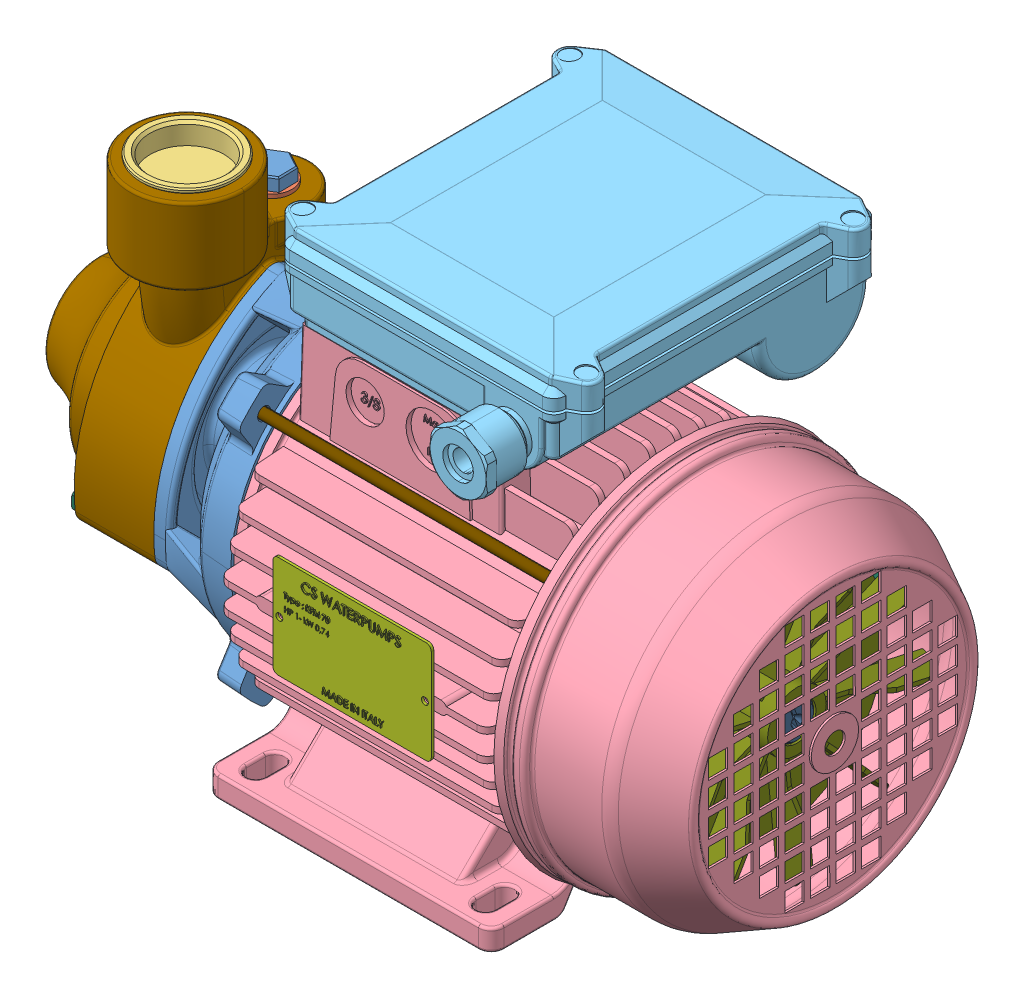
SolidWorks assembly Elettropompa KF  Inox, configuration Default. Lengths in mm.
Overall size (290.35 207.83 196.66).
68 component instances, 35 part files, 71 mates.
Components (placement in the parent):
- Supporto motore KF 65_70-1: Supporto motore KF 65_70 [Default] at (-54.2626 10.5524 119.1659) x (0 0 1) z (-1 0 0) size (120 120 55)
- Gruppo statore avvolto H80 con carcassa  B3 e portacondensatore-1: Gruppo statore avvolto H80 con carcassa  B3 e portacondensatore [Default] at (62.7261 5.2741 9.1659) size (151.55 207.83 196.66)
  - Statore 110x55H70-1: Statore 110x55H70 [Default] at (-35.1887 5.2783 110) x (0 0 -1) z (1 0 0) size (110 110 80)
  - corona avvolgimeno-1: corona avvolgimeno [Default] at (-75.1887 5.2783 110) x (0 -0.91858 0.395234) z (0 -0.395234 -0.91858) size (95 25 95)
  - corona avvolgimeno-2: corona avvolgimeno [Default] at (4.8113 5.2783 110) x (0 0.057001 0.998374) z (0 0.998374 -0.057001) size (95 25 95)
  - Carcassa MEC 71 B3-1: Carcassa MEC 71 B3 [Default] at (14.0613 5.2783 110) x (0 0 1) z (-1 0 0) size (140 148 121.5)
  - COPRIMORS_MEC63-71_MONOFASE_M4-1: COPRIMORS_MEC63-71_MONOFASE_M4 [Default] at (-55.6887 85.2783 110) x (-1 0 0) z (0 0 -1) size (121.11 50.5 148)
  - Calotta MEC 71 Lavorata-1: Calotta MEC 71 Lavorata [Default] at (15.8113 5.2783 110) x (0 -0.70802 -0.706193) z (0 -0.706193 0.70802) size (139.06 30 139.06)
  - targhetta metallica-1: targhetta metallica [Default] at (-10.1875 -9.7179 181) x (-1 -0.000063 0) z (0 0 -1) size (62 40 1.5)
- Girante cod KFM 65_70-1: Girante cod KFM 65_70 [Default] at (-95.8876 10.5524 119.1659) x (0 0.937754 0.347301) z (-1 0 0) size (70.8 70.8 15.13)
- Corpo pompa KF 65_70-1: Corpo pompa KF 65_70 [Default] at (-96.0626 10.5524 119.1659) x (0 0 1) z (-1 0 0) size (93.39 132.5 74.65)
- Assieme9-1: Assieme9 [Default] at (49.0791 -228.781 32.0447) x (1 0 0) z (0 0.937754 0.347301) size (231.8 61.88 61.88)
  - Albero KF 70-1: Albero KF 70 [Default] at (75.6583 1.4226 254.6931) x (-1 0 0) z (0 0 -1) size (231.8 17 17)
  - SKF_W_6202_2RS1-1: SKF_W_6202_2RS1 [Default] at (38.6583 1.4226 254.6931) x (1 0 0) z (0 -0.991359 0.13118) size (11 35 35)
    - SKF_W_6202_2RS1_12-1: SKF_W_6202_2RS1_12 [Default] x (1 0 0) z (0 -0.707107 0.707107) size (5.95 5.95 5.95)
    - SKF_W_6202_2RS1_12-2: SKF_W_6202_2RS1_12 [Default] x (1 0 0) z (0 -1 0) size (5.95 5.95 5.95)
    - SKF_W_6202_2RS1_12-3: SKF_W_6202_2RS1_12 [Default] x (1 0 0) z (0 -0.707107 -0.707107) size (5.95 5.95 5.95)
    - SKF_W_6202_2RS1_12-4: SKF_W_6202_2RS1_12 [Default] x (1 0 0) z (0 0 -1) size (5.95 5.95 5.95)
    - SKF_W_6202_2RS1_12-5: SKF_W_6202_2RS1_12 [Default] x (1 0 0) z (0 0.707107 -0.707107) size (5.95 5.95 5.95)
    - SKF_W_6202_2RS1_12-6: SKF_W_6202_2RS1_12 [Default] x (1 0 0) z (0 1 0) size (5.95 5.95 5.95)
    - SKF_W_6202_2RS1_12-7: SKF_W_6202_2RS1_12 [Default] x (1 0 0) z (0 0.707107 0.707107) size (5.95 5.95 5.95)
    - SKF_W_6202_2RS1_12-8: SKF_W_6202_2RS1_12 [Default] at origin size (5.95 5.95 5.95)
    - SKF_W_6202_2RS1_21-1: SKF_W_6202_2RS1_21 [Default] at origin size (11 35 35)
    - SKF_W_6202_2RS1_23-1: SKF_W_6202_2RS1_23 [Default] at origin size (11 31.4 31.4)
  - SKF_W_6202_2RS1-2: SKF_W_6202_2RS1 [Default] at (-103.3417 1.4226 254.6931) x (1 0 0) z (0 -0.849888 -0.526963) size (11 35 35)
    - SKF_W_6202_2RS1_12-1: SKF_W_6202_2RS1_12 [Default] x (1 0 0) z (0 -0.707107 0.707107) size (5.95 5.95 5.95)
    - SKF_W_6202_2RS1_12-2: SKF_W_6202_2RS1_12 [Default] x (1 0 0) z (0 -1 0) size (5.95 5.95 5.95)
    - SKF_W_6202_2RS1_12-3: SKF_W_6202_2RS1_12 [Default] x (1 0 0) z (0 -0.707107 -0.707107) size (5.95 5.95 5.95)
    - SKF_W_6202_2RS1_12-4: SKF_W_6202_2RS1_12 [Default] x (1 0 0) z (0 0 -1) size (5.95 5.95 5.95)
    - SKF_W_6202_2RS1_12-5: SKF_W_6202_2RS1_12 [Default] x (1 0 0) z (0 0.707107 -0.707107) size (5.95 5.95 5.95)
    - SKF_W_6202_2RS1_12-6: SKF_W_6202_2RS1_12 [Default] x (1 0 0) z (0 1 0) size (5.95 5.95 5.95)
    - SKF_W_6202_2RS1_12-7: SKF_W_6202_2RS1_12 [Default] x (1 0 0) z (0 0.707107 0.707107) size (5.95 5.95 5.95)
    - SKF_W_6202_2RS1_12-8: SKF_W_6202_2RS1_12 [Default] at origin size (5.95 5.95 5.95)
    - SKF_W_6202_2RS1_21-1: SKF_W_6202_2RS1_21 [Default] at origin size (11 35 35)
    - SKF_W_6202_2RS1_23-1: SKF_W_6202_2RS1_23 [Default] at origin size (11 31.4 31.4)
  - Rotore-1: Rotore [90] at (-20.3417 1.4226 254.6931) x (1 0 0) z (0 -0.148651 0.98889) size (88 54.4 54.4)
  - Chiavetta 4x4x10-1: Chiavetta 4x4x10 [Default] at (-148.1417 8.4226 254.6931) x (1 0 0) z (0 -1 0) size (10 4 3.8)
- Ventola MEC71  FORO 15-1: Ventola MEC71  FORO 15 [Default] at (-99.6626 10.5524 119.1659) x (0 -0.861898 0.507081) z (1 0 0) size (127 121.28 15.42)
- Rompigoccia-1: Rompigoccia [Default] at (-54.2626 10.5524 119.1659) x (0 0 1) z (0 -1 0) size (33.06 8 33.06)
- tirante  5x135-1: tirante  5x135 [Default] at (86.5374 55.5524 164.1659) x (-1 0 0) z (0 0 -1) size (137.41 8.1 7.02)
- tirante  5x135-2: tirante  5x135 [Default] at (86.5374 -34.4476 164.1659) x (-1 0 0) z (0 -0.8306 -0.556869) size (137.41 8.1 7.02)
- tirante  5x135-3: tirante  5x135 [Default] at (86.5374 55.5524 74.1659) x (-1 0 0) z (0 -0.008382 -0.999965) size (137.41 8.1 7.02)
- tirante  5x135-4: tirante  5x135 [Default] at (86.5374 -34.4476 74.1659) x (-1 0 0) z (0 -0.959675 -0.281111) size (137.41 8.1 7.02)
- tappo 1_8-1: tappo 1_8 [Default] at (-96.0626 77.0524 104.1659) x (-1 0 0) z (0 1 0) size (13.16 15.01 12)
- Rondella alluminio 1_8-1: Rondella alluminio 1_8 [Default] at (-96.0626 75.5524 104.1659) size (16 1.5 16)
- Tappo salvafiletto 1 pollice-1: Tappo salvafiletto 1 pollice [Default] at (-140.7406 10.5524 119.1659) x (-1 0 0) z (0 0.938506 0.345262) size (9.54 36.1 36.1)
- Tappo salvafiletto 1 pollice-2: Tappo salvafiletto 1 pollice [Default] at (-96.0626 92.8304 137.1659) x (0 1 0) z (0.026176 0 -0.999657) size (9.54 36.1 36.1)
- Copriventola MEC 71-1: Copriventola MEC 71 [Default] at (77.5374 10.5524 119.1659) x (-1 0 0) z (0 -0.000219 1) size (62.53 143.02 143.02)
- morsettiera-1: morsettiera [Default] at (30.5627 41.122 115.2906) x (0 0 1) z (0 1 0) size (27 42 19.32)
  - base morsettiera-1: base morsettiera [Default] at (3.8753 -23.6462 42.9304) x (-1 0 0) z (0 0 -1) size (27 42 10.5)
  - perno morsettiera-1: perno morsettiera [Default] at (11.8753 -39.1462 42.6304) size (4.5 4.63 11.12)
  - perno morsettiera-2: perno morsettiera [Default] at (-4.1247 -39.1462 42.6304) size (4.5 4.63 11.12)
  - perno morsettiera-3: perno morsettiera [Default] at (11.8753 -8.1462 42.6304) size (4.5 4.63 11.12)
- STAZIONARIA-2: STAZIONARIA [Default] at (-71.4228 -14.1935 127.8022) x (0 -0.44605 -0.895008) z (0 0.895008 -0.44605) size (26 8 26)
  - GOMMA-1: GOMMA [Default] at (-3.3084 -4.4601 26) size (26 7 26)
  - CERAMICA-1: CERAMICA [Default] at (-3.3084 -0.9601 26) x (0.999975 0 0.00709) z (-0.00709 0 0.999975) size (22 4.5 22)
- ROTANTE-1: ROTANTE [Default] at (-75.2954 30.2911 126.3816) x (0 -0.30619 0.951971) z (0 -0.951971 -0.30619) size (32.11 13 32.11)
  - Parte4-1: Parte4 [Default] at (-0.8254 8.0815 21) size (21 3.5 21)
  - Parte5-1: Parte5 [Default] at (-0.8254 1.4673 21) size (24 8.4 24)
  - Parte6-1: Parte6 [Default] at (-0.8254 -0.3327 21) size (23 5 23)
  - Parte7-1: Parte7 [Default] at (-0.8254 4.6673 21) size (23 8 23)
  - Parte8-1: Parte8 [Default] at (-0.8254 5.6673 21) x (0.584934 0 0.811081) z (-0.811081 0 0.584934) size (23 1 23)
  - Parte2-2: Parte2 [Default] at (-0.5063 7.2427 20.915) x (-1 0 0) z (0 1 0) size (21.2 21.25 5.09)
- 621015x35-1: 621015x35 [Default] at (-111.6626 57.0524 119.1659) size (38.51 9.26 8.02)
- 621015x35-2: 621015x35 [Default] at (-111.6626 -12.6976 159.4361) size (38.51 9.26 8.02)
- 621015x35-3: 621015x35 [Default] at (-111.6626 -12.6976 78.8957) size (38.51 9.26 8.02)
- 10_00_0471_0120_002-1: 10_00_0471_0120_002 [Default] at (-89.0626 10.46 119.5551) x (0 -0.972953 -0.231005) z (1 0 0) size (14.3 16.3 1)
- Rondella tenuta-1: Rondella tenuta [Default] at (-88.0626 10.5524 119.1659) x (0 0 -1) z (0 -1 0) size (21 0.1 21)
Mates (geometry in assembly coordinates):
- Concentrico1: concentric aligned: cylinder of Supporto motore KF 65_70-1 through (-54.2626 10.5524 119.1659) axis (1 0 0) radius 56.9; cylinder of Gruppo statore avvolto H80 con carcassa  B3 e portacondensatore-1/Carcassa MEC 71 B3-1 through (-39.9626 10.5524 119.1659) axis (1 0 0) radius 57
- Coincidente1: coincident anti-aligned: plane of Supporto motore KF 65_70-1 through (-36.9626 67.4524 119.1659) normal (1 0 0); plane of Gruppo statore avvolto H80 con carcassa  B3 e portacondensatore-1/Carcassa MEC 71 B3-1 through (-36.9626 10.5524 119.1659) normal (-1 0 0)
- Concentrico2: concentric anti-aligned: circle of Supporto motore KF 65_70-1; circle of Girante cod KFM 65_70-1
- Distanza1: distance = 0.05 mm anti-aligned: plane of Girante cod KFM 65_70-1 through (-92.0126 18.9571 96.4723) normal (1 0 0); plane of Supporto motore KF 65_70-1 through (-91.9626 35.7524 119.1659) normal (-1 0 0)
- Concentrico3: concentric aligned: cylinder of Supporto motore KF 65_70-1 through (-54.2626 10.5524 119.1659) axis (1 0 0) radius 35.45; cylinder of Corpo pompa KF 65_70-1 through (-104.2626 10.5524 119.1659) axis (1 0 0) radius 35.5
- Coincidente3: coincident anti-aligned: plane of Supporto motore KF 65_70-1 through (-80.4626 63.0524 119.1659) normal (-1 0 0); plane of Corpo pompa KF 65_70-1 through (-80.4626 -8.9027 125.7387) normal (1 0 0)
- Coincidente4: coincident anti-aligned: plane of Supporto motore KF 65_70-1 through (-54.2626 23.0524 119.1659) normal (1 0 0); plane of Assieme9-1/SKF_W_6202_2RS1-2/SKF_W_6202_2RS1_21-1 through (-54.2626 20.9285 132.5055) normal (-1 0 0)
- Concentrico4: concentric aligned: cylinder of Supporto motore KF 65_70-1 through (-54.2626 10.5524 119.1659) axis (1 0 0) radius 17.5; cylinder of Assieme9-1/SKF_W_6202_2RS1-2/SKF_W_6202_2RS1_21-1 through (-4.2626 10.5524 119.1659) axis (1 0 0) radius 17.5
- Coincidente5: coincident anti-aligned: plane of Girante cod KFM 65_70-1 through (-92.0126 11.4727 110.9224) normal (0 0.937754 0.347301); plane of Assieme9-1/Chiavetta 4x4x10-1 through (-102.0626 9.7883 115.4705) normal (0 -0.937754 -0.347301)
- Concentrico5: concentric aligned: circle of Gruppo statore avvolto H80 con carcassa  B3 e portacondensatore-1/Calotta MEC 71 Lavorata-1; cylinder of Ventola MEC71  FORO 15-1 through (124.7374 10.5524 119.1659) axis (1 0 0) radius 7.5
- Coincidente6: coincident aligned: plane of Assieme9-1/Albero KF 70-1 through (124.7374 10.5524 119.1659) normal (1 0 0); plane of Ventola MEC71  FORO 15-1 through (124.7374 10.5524 119.1659) normal (1 0 0)
- Blocca1: lock: unknown of Assieme9-1/Albero KF 70-1; unknown of Ventola MEC71  FORO 15-1
- Concentrico6: concentric anti-aligned: cylinder of Assieme9-1/Albero KF 70-1 through (124.7374 10.5524 119.1659) axis (1 0 0) radius 6; cylinder of Rompigoccia-1 through (-97.7632 10.5524 119.1659) axis (-1 0 0) radius 6
- Coincidente7: coincident anti-aligned: plane of Assieme9-1/Albero KF 70-1 through (-54.2626 12.6363 113.5394) normal (-1 0 0); plane of Rompigoccia-1 through (-54.2626 10.5524 113.1659) normal (1 0 0)
- Concentrico7: concentric anti-aligned: cylinder of Supporto motore KF 65_70-1 through (-38.9626 55.5524 164.1659) axis (1 0 0) radius 2.1; cylinder of tirante  5x135-1 through (86.9374 55.5524 164.1659) axis (-1 0 0) radius 2
- Coincidente8: coincident anti-aligned: plane of Gruppo statore avvolto H80 con carcassa  B3 e portacondensatore-1/Calotta MEC 71 Lavorata-1 through (86.5374 59.7806 168.267) normal (1 0 0); plane of tirante  5x135-1 through (86.5374 57.5524 164.1659) normal (-1 0 0)
- Concentrico8: concentric anti-aligned: cylinder of Supporto motore KF 65_70-1 through (-38.9626 -34.4476 164.1659) axis (1 0 0) radius 2.1; cylinder of tirante  5x135-2 through (86.9374 -34.4476 164.1659) axis (-1 0 0) radius 2
- Coincidente10: coincident anti-aligned: plane of Gruppo statore avvolto H80 con carcassa  B3 e portacondensatore-1/Calotta MEC 71 Lavorata-1 through (86.5374 -38.5487 168.3941) normal (1 0 0); plane of tirante  5x135-2 through (86.5374 -33.3338 162.5047) normal (-1 0 0)
- Concentrico9: concentric anti-aligned: cylinder of Supporto motore KF 65_70-1 through (-38.9626 55.5524 74.1659) axis (1 0 0) radius 2.1; cylinder of tirante  5x135-3 through (86.9374 55.5524 74.1659) axis (-1 0 0) radius 2
- Coincidente11: coincident anti-aligned: plane of Gruppo statore avvolto H80 con carcassa  B3 e portacondensatore-1/Calotta MEC 71 Lavorata-1 through (86.5374 59.6536 69.9377) normal (1 0 0); plane of tirante  5x135-3 through (86.5374 57.5524 74.1491) normal (-1 0 0)
- Concentrico10: concentric anti-aligned: cylinder of Supporto motore KF 65_70-1 through (-38.9626 -34.4476 74.1659) axis (1 0 0) radius 2.1; cylinder of tirante  5x135-4 through (86.9374 -34.4476 74.1659) axis (-1 0 0) radius 2
- Coincidente12: coincident anti-aligned: plane of Gruppo statore avvolto H80 con carcassa  B3 e portacondensatore-1/Calotta MEC 71 Lavorata-1 through (86.5374 -38.6758 70.0647) normal (1 0 0); plane of tirante  5x135-4 through (86.5374 -33.8853 72.2465) normal (-1 0 0)
- Parallelo2: parallel anti-aligned: plane of Gruppo statore avvolto H80 con carcassa  B3 e portacondensatore-1/Carcassa MEC 71 B3-1 through (-36.9626 -59.4476 74.3349) normal (0 -1 0); plane of Corpo pompa KF 65_70-1 through (-96.0626 100.5524 137.1659) normal (0 1 0)
- Concentrico121: concentric anti-aligned: cylinder of Corpo pompa KF 65_70-1 through (-111.6626 57.0524 119.1659) axis (1 0 0) radius 2.75; cylinder of hex bolt gradeab_iso-1 through (-115.1626 57.0495 118.6437) axis (-1 0 0) radius 4
- Coincidente141: coincident anti-aligned: plane of Corpo pompa KF 65_70-1 through (-111.6626 -8.9027 125.7387) normal (-1 0 0); plane of hex bolt gradeab_iso-1 through (-111.6626 61.6683 118.6437) normal (1 0 0)
- Concentrico13: concentric anti-aligned: cylinder of Corpo pompa KF 65_70-1 through (-111.6626 -12.6976 159.4361) axis (1 0 0) radius 2.75; cylinder of hex bolt gradeab_iso-2 through (-115.1626 -10.3429 160.7067) axis (-1 0 0) radius 4
- Coincidente15: coincident anti-aligned: plane of Corpo pompa KF 65_70-1 through (-111.6626 -8.9027 125.7387) normal (-1 0 0); plane of hex bolt gradeab_iso-2 through (-111.6626 -5.7241 160.7067) normal (1 0 0)
- Concentrico14: concentric anti-aligned: cylinder of Corpo pompa KF 65_70-1 through (-111.6626 -12.6976 78.8957) axis (1 0 0) radius 6; cylinder of hex bolt gradeab_iso-3 through (-115.1626 -14.9753 80.2996) axis (-1 0 0) radius 4
- Coincidente16: coincident anti-aligned: plane of Corpo pompa KF 65_70-1 through (-111.6626 -8.9027 125.7387) normal (-1 0 0); plane of hex bolt gradeab_iso-3 through (-111.6626 -10.3565 80.2996) normal (1 0 0)
- Concentrico15: concentric anti-aligned: cylinder of Corpo pompa KF 65_70-1 through (-111.6626 57.0524 119.1659) axis (1 0 0) radius 2.75; cylinder of hex bolt gradeab_iso-4 through (-115.1626 56.9755 116.4914) axis (-1 0 0) radius 4
- Coincidente17: coincident anti-aligned: plane of Corpo pompa KF 65_70-1 through (-111.6626 -8.9027 125.7387) normal (-1 0 0); plane of hex bolt gradeab_iso-4 through (-111.6626 61.5943 116.4914) normal (1 0 0)
- Concentrico16: concentric anti-aligned: cylinder of Corpo pompa KF 65_70-1 through (-111.6626 -12.6976 159.4361) axis (1 0 0) radius 2.75; cylinder of hex bolt gradeab_iso-5 through (-115.1626 -10.3429 160.7067) axis (-1 0 0) radius 4
- Coincidente18: coincident anti-aligned: plane of Corpo pompa KF 65_70-1 through (-111.6626 -8.9027 125.7387) normal (-1 0 0); plane of hex bolt gradeab_iso-5 through (-111.6626 -5.7241 160.7067) normal (1 0 0)
- Concentrico17: concentric: cylinder of Corpo pompa KF 65_70-1 through (-111.6626 -12.6976 78.8957) axis (1 0 0) radius 2.75; cylinder of hex bolt gradeab_iso-6 through (-115.1626 -14.9753 80.2996) axis (-1 0 0) radius 4
- Coincidente19: coincident anti-aligned: plane of Corpo pompa KF 65_70-1 through (-111.6626 -8.9027 125.7387) normal (-1 0 0); plane of hex bolt gradeab_iso-6 through (-111.6626 -10.3565 80.2996) normal (1 0 0)
- Concentrico18: concentric anti-aligned: cylinder of Corpo pompa KF 65_70-1 through (-111.6626 57.0524 119.1659) axis (1 0 0) radius 2.75; cylinder of hex bolt gradeab_iso-7 through (-115.1626 57.0524 119.1659) axis (-1 0 0) radius 4
- Coincidente20: coincident anti-aligned: plane of Corpo pompa KF 65_70-1 through (-111.6626 -8.9027 125.7387) normal (-1 0 0); plane of hex bolt gradeab_iso-7 through (-111.6626 61.1206 116.9788) normal (1 0 0)
- Concentrico19: concentric anti-aligned: cylinder of Corpo pompa KF 65_70-1 through (-111.6626 -12.6976 159.4361) axis (1 0 0) radius 6; cylinder of hex bolt gradeab_iso-8 through (-115.1626 -12.6976 159.4361) axis (-1 0 0) radius 4
- Coincidente21: coincident anti-aligned: plane of Corpo pompa KF 65_70-1 through (-111.6626 -8.9027 125.7387) normal (-1 0 0); plane of hex bolt gradeab_iso-8 through (-111.6626 -8.0788 159.4361) normal (1 0 0)
- Concentrico20: concentric anti-aligned: cylinder of Corpo pompa KF 65_70-1 through (-111.6626 -12.6976 78.8957) axis (1 0 0) radius 2.75; cylinder of hex bolt gradeab_iso-9 through (-115.1626 -12.6976 78.8957) axis (-1 0 0) radius 4
- Coincidente22: coincident anti-aligned: plane of Corpo pompa KF 65_70-1 through (-111.6626 -8.9027 125.7387) normal (-1 0 0); plane of hex bolt gradeab_iso-9 through (-111.6626 -8.0788 78.8957) normal (1 0 0)
- Concentrico26: concentric aligned: cylinder of Supporto motore KF 65_70-1 through (-80.4626 57.0524 119.1659) axis (-1 0 0) radius 2.1; cylinder of hex bolt gradeab_iso-7 through (-115.1626 57.0524 119.1659) axis (-1 0 0) radius 2.5
- Coincidente23: coincident anti-aligned: plane of Corpo pompa KF 65_70-1 through (-96.0626 75.5524 104.1659) normal (0 1 0); plane of Rondella alluminio 1_8-1 through (-96.0626 75.5524 104.1659) normal (0 -1 0)
- Concentrico28: concentric aligned: cylinder of Corpo pompa KF 65_70-1 through (-96.0626 75.5524 104.1659) axis (0 1 0) radius 4.25; cylinder of Rondella alluminio 1_8-1 through (-96.0626 75.5524 104.1659) axis (0 1 0) radius 5
- Coincidente24: coincident anti-aligned: plane of tappo 1_8-1 through (-96.0626 77.0524 104.1659) normal (0 -1 0); plane of Rondella alluminio 1_8-1 through (-96.0626 77.0524 104.1659) normal (0 1 0)
- Concentrico29: concentric aligned: cylinder of Corpo pompa KF 65_70-1 through (-96.0626 75.5524 104.1659) axis (0 1 0) radius 4.25; cylinder of tappo 1_8-1 through (-96.0626 70.0524 104.1659) axis (0 1 0) radius 4.8
- Concentrico30: concentric aligned: cylinder of Corpo pompa KF 65_70-1 through (-148.4626 10.5524 119.1659) axis (-1 0 0) radius 15.375; cylinder of Tappo salvafiletto 1 pollice-1 through (-142.0406 10.5524 119.1659) axis (-1 0 0) radius 15.5
- Coincidente25: coincident anti-aligned: plane of Corpo pompa KF 65_70-1 through (-148.4626 32.0524 119.1659) normal (-1 0 0); plane of Tappo salvafiletto 1 pollice-1 through (-148.4626 5.2009 133.7127) normal (1 0 0)
- Concentrico31: concentric aligned: cylinder of Corpo pompa KF 65_70-1 through (-96.0626 100.5524 137.1659) axis (0 1 0) radius 15.375; cylinder of Tappo salvafiletto 1 pollice-2 through (-96.0626 94.1304 137.1659) axis (0 1 0) radius 15.5
- Coincidente26: coincident anti-aligned: plane of Corpo pompa KF 65_70-1 through (-96.0626 100.5524 137.1659) normal (0 1 0); plane of Tappo salvafiletto 1 pollice-2 through (-80.5679 100.5524 137.5716) normal (0 -1 0)
- Concentrico32: concentric aligned: circle of Gruppo statore avvolto H80 con carcassa  B3 e portacondensatore-1/Carcassa MEC 71 B3-1; circle of Copriventola MEC 71-1
- Distanza2: distance = 1 mm aligned: plane of Gruppo statore avvolto H80 con carcassa  B3 e portacondensatore-1/Calotta MEC 71 Lavorata-1 through (78.5374 10.5524 119.1659) normal (-1 0 0); plane of Copriventola MEC 71-1 through (77.5374 -60.959 119.1502) normal (-1 0 0)
- Coincidente28: coincident anti-aligned: plane of Gruppo statore avvolto H80 con carcassa  B3 e portacondensatore-1/Carcassa MEC 71 B3-1 through (-3.7718 75.5524 119.1659) normal (0 1 0); plane of morsettiera-1/base morsettiera-1 through (24.9165 75.5524 129.6659) normal (0 -1 0)
- Concentrico33: concentric aligned: circle of Gruppo statore avvolto H80 con carcassa  B3 e portacondensatore-1/Carcassa MEC 71 B3-1; circle of morsettiera-1/base morsettiera-1
- Parallelo5: parallel anti-aligned: plane of Gruppo statore avvolto H80 con carcassa  B3 e portacondensatore-1/Carcassa MEC 71 B3-1 through (41.5374 -65.4486 86.1659) normal (-1 0 0); plane of morsettiera-1/base morsettiera-1 through (27.9165 75.5524 129.6659) normal (1 0 0)
- Concentrico122: concentric anti-aligned: cylinder of Supporto motore KF 65_70-1 through (-54.2626 10.5524 119.1659) axis (1 0 0) radius 13; cylinder of STAZIONARIA-1/GOMMA-1 through (-79.3822 10.5524 119.1659) axis (-1 0 0) radius 13
- Concentrico123: concentric anti-aligned: cylinder of Supporto motore KF 65_70-1 through (-54.2626 10.5524 119.1659) axis (1 0 0) radius 13; cylinder of STAZIONARIA-2/GOMMA-1 through (-104.9108 10.5524 119.1659) axis (-1 0 0) radius 13
- Coincidente142: coincident anti-aligned: plane of Supporto motore KF 65_70-1 through (-66.9626 18.2024 119.1659) normal (-1 0 0); plane of STAZIONARIA-2/GOMMA-1 through (-66.9626 13.8978 125.8784) normal (1 0 0)
- Concentrico124: concentric anti-aligned: cylinder of Assieme9-1/Albero KF 70-1 through (124.7374 10.5524 119.1659) axis (1 0 0) radius 6; cylinder of ROTANTE-1/Parte7-1 through (-106.8855 10.5524 119.1659) axis (-1 0 0) radius 6
- Coincidente143: coincident anti-aligned: plane of STAZIONARIA-2/CERAMICA-1 through (-74.9626 15.2572 128.7761) normal (-1 0 0); plane of ROTANTE-1/Parte6-1 through (-74.9626 12.9101 111.8357) normal (1 0 0)
- Concentrico126: concentric anti-aligned: cylinder of Supporto motore KF 65_70-1 through (-80.4626 57.0524 119.1659) axis (-1 0 0) radius 2.1; cylinder of 621015x35-1 through (-76.6626 57.0524 119.1659) axis (1 0 0) radius 2.5
- Concentrico127: concentric anti-aligned: circle of Corpo pompa KF 65_70-1; cylinder of 621015x35-1 through (-76.6626 57.0524 119.1659) axis (1 0 0) radius 2.5
- Coincidente144: coincident anti-aligned: plane of Corpo pompa KF 65_70-1 through (-111.6626 -8.9027 125.7387) normal (-1 0 0); plane of 621015x35-1 through (-111.6626 60.4924 119.1659) normal (1 0 0)
- Concentrico128: concentric aligned: cylinder of Corpo pompa KF 65_70-1 through (-111.6626 -12.6976 159.4361) axis (1 0 0) radius 2.75; cylinder of 621015x35-2 through (-76.6626 -12.6976 159.4361) axis (1 0 0) radius 2.5
- Coincidente145: coincident anti-aligned: plane of Corpo pompa KF 65_70-1 through (-111.6626 -8.9027 125.7387) normal (-1 0 0); plane of 621015x35-2 through (-111.6626 -9.2576 159.4361) normal (1 0 0)
- Concentrico129: concentric aligned: cylinder of Corpo pompa KF 65_70-1 through (-111.6626 -12.6976 78.8957) axis (1 0 0) radius 2.75; cylinder of 621015x35-3 through (-76.6626 -12.6976 78.8957) axis (1 0 0) radius 2.5
- Coincidente146: coincident anti-aligned: plane of Corpo pompa KF 65_70-1 through (-111.6626 -8.9027 125.7387) normal (-1 0 0); plane of 621015x35-3 through (-111.6626 -9.2576 78.8957) normal (1 0 0)
- Concentrico130: concentric aligned: cylinder of Assieme9-1/Albero KF 70-1 through (124.7374 10.5524 119.1659) axis (1 0 0) radius 5.3891; cylinder of 10_00_0471_0120_002-1 through (-88.5626 10.5524 119.1659) axis (1 0 0) radius 5.75
- Coincidente147: coincident anti-aligned: plane of Assieme9-1/Albero KF 70-1 through (-88.0626 12.4241 114.1123) normal (-1 0 0); plane of 10_00_0471_0120_002-1 through (-88.0626 7.661 118.1073) normal (1 0 0)
- Coincidente148: coincident aligned: cylinder of Assieme9-1/Albero KF 70-1 through (124.7374 10.5524 119.1659) axis (1 0 0) radius 6; circle of Rondella tenuta-1
- Coincidente149: coincident anti-aligned: plane of ROTANTE-1/Parte7-1 through (-87.9626 13.0785 111.3121) normal (-1 0 0); plane of Rondella tenuta-1 through (-87.9626 10.5524 129.6659) normal (1 0 0)
